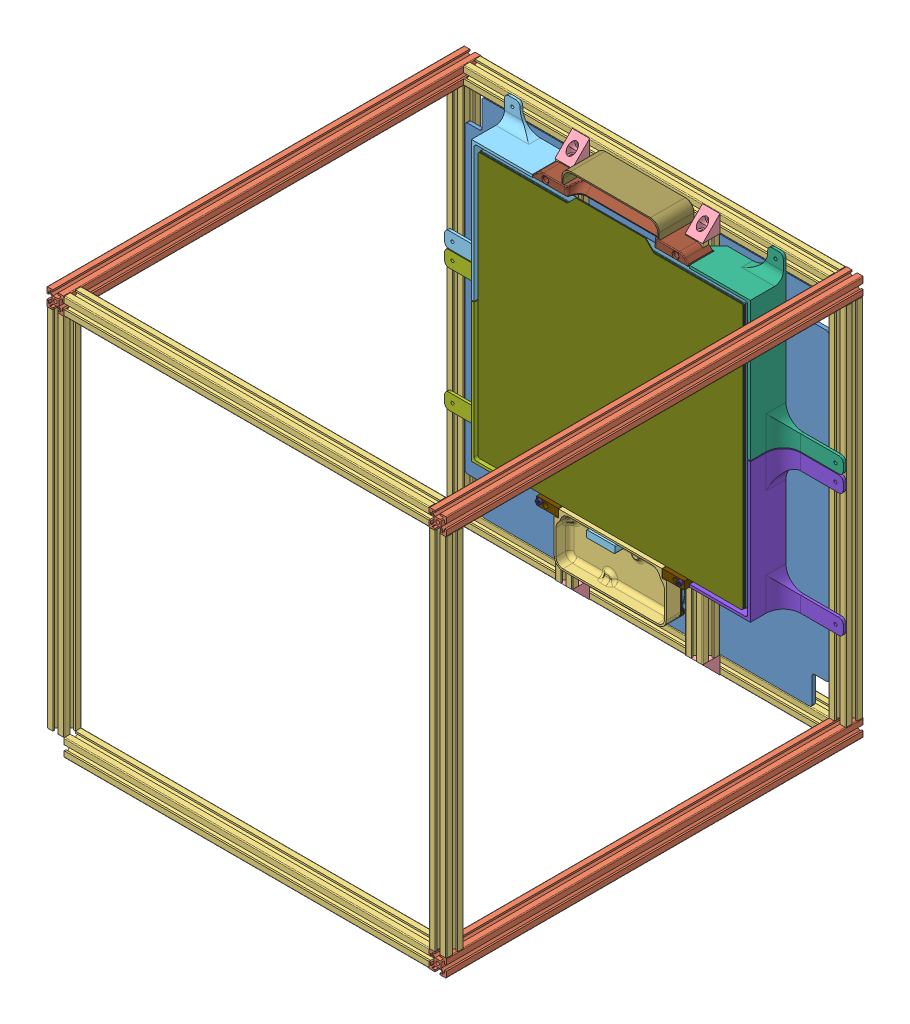
SolidWorks assembly Voron_full, configuration Default. Lengths in mm.
Overall size (460 460 480).
60 component instances, 23 part files, 98 mates.
Components (placement in the parent):
- bottom panel-1: bottom panel [Default] at (79.6442 547.5398 47.79) size (419 419 4)
- Misumi HFSB5-2020-480-1: Misumi HFSB5-2020-480 [Default] at (298.6442 327.5398 271.79) x (1 0 0) z (0 -1 0) size (20 480 20)
- Misumi HFSB5-2020-480-2: Misumi HFSB5-2020-480 [Default] at (-141.3558 327.5398 271.79) x (1 0 0) z (0 -1 0) size (20 480 20) (hidden)
- Misumi HFSB5-2020-480-3: Misumi HFSB5-2020-480 [Default] at (298.6442 767.5398 271.79) x (1 0 0) z (0 -1 0) size (20 480 20)
- Misumi HFSB5-2020-480-4: Misumi HFSB5-2020-480 [Default] at (-141.3558 767.5398 271.79) x (1 0 0) z (0 -1 0) size (20 480 20)
- Misumi HFSB5-2020-420-6: Misumi HFSB5-2020-420 [Default] at (-141.3558 547.5398 41.79) size (20 420 20)
- Misumi HFSB5-2020-420-8: Misumi HFSB5-2020-420 [Default] at (298.6442 547.5398 41.79) size (20 420 20)
- Misumi HFSB5-2020-420-10: Misumi HFSB5-2020-420 [Default] at (78.6442 327.5398 41.79) x (0 1 0) z (0 0 1) size (20 420 20)
- Misumi HFSB5-2020-420-12: Misumi HFSB5-2020-420 [Default] at (78.6442 767.5398 41.79) x (0 1 0) z (0 0 1) size (20 420 20)
- Misumi HFSB5-2020-420-7: Misumi HFSB5-2020-420 [Default] at (-141.3558 547.5398 501.79) size (20 420 20)
- Misumi HFSB5-2020-420-9: Misumi HFSB5-2020-420 [Default] at (298.6442 547.5398 501.79) size (20 420 20)
- Misumi HFSB5-2020-420-11: Misumi HFSB5-2020-420 [Default] at (78.6442 327.5398 501.79) x (0 1 0) z (0 0 1) size (20 420 20)
- Misumi HFSB5-2020-420-13: Misumi HFSB5-2020-420 [Default] at (78.6442 767.5398 501.79) x (0 1 0) z (0 0 1) size (20 420 20)
- Misumi HFSB5-2020-420-14: Misumi HFSB5-2020-420 [Default] at (153.6442 547.5398 61.79) size (20 420 20)
- Misumi HFSB5-2020-420-15: Misumi HFSB5-2020-420 [Default] at (3.6442 547.5398 61.79) size (20 420 20)
- OpenBuilds Billet Angle Corner Connector (2020)-1: OpenBuilds Billet Angle Corner Connector (2020) [Default] at (3.6442 757.5398 51.79) size (20 20 20)
- OpenBuilds Billet Angle Corner Connector (2020)-2: OpenBuilds Billet Angle Corner Connector (2020) [Default] at (153.6442 757.5398 51.79) size (20 20 20)
- OpenBuilds Billet Angle Corner Connector (2020)-3: OpenBuilds Billet Angle Corner Connector (2020) [Default] at (3.6442 337.5398 51.79) x (-1 0 0) z (0 0 1) size (20 20 20)
- OpenBuilds Billet Angle Corner Connector (2020)-4: OpenBuilds Billet Angle Corner Connector (2020) [Default] at (153.6442 337.5398 51.79) x (-1 0 0) z (0 0 1) size (20 20 20)
- Draft nozzle front side 1-3: Draft nozzle front side 1 [Default] at (-43.8558 669.5398 51.79) x (0 -1 0) z (0 0 1) size (187 149.5 41)
- Draft nozzle front side 2-2: Draft nozzle front side 2 [Default] at (277.1442 669.5398 51.79) x (0 -1 0) z (0 0 1) size (187 149.5 41)
- Draft nozzle back side 1-1: Draft nozzle back side 1 [Default] at (-43.8558 668.5398 51.79) x (0 -1 0) z (0 0 1) size (160 149.5 41)
- Draft nozzle back side 2-1: Draft nozzle back side 2 [Default] at (277.1442 668.5398 51.79) x (0 -1 0) z (0 0 1) size (160 149.5 41)
- Z-Stop LDO Mirrored-1: Z-Stop LDO Mirrored [Default] at (-16.3558 430.0398 68.79) x (0 1 0) z (0 0 -1) size (35 20.8 15.3)
- inner draft shield-1: inner draft shield [Default] at (78.6442 661.5398 51.79) x (-1 0 0) z (0 0 1) size (129 20 22)
- Draft nozzle front-3: Draft nozzle front [Default] at (78.6442 746.5398 72.04) x (-1 0 0) z (0 1 0) size (179 41.54 13.26)
- front_bucket-1: front_bucket [Default] at (78.6442 764.0398 51.79) x (-1 0 0) z (0 0 1) size (112 21 41)
- knurled nut-1: knurled nut [Default] at (154.1442 443.5398 73.7694) size (16 16 9.5)
- knurled nut-2: knurled nut [Default] at (154.1442 734.5398 73.7694) size (16 16 9.5)
- knurled nut-3: knurled nut [Default] at (4.1442 734.5398 73.7694) size (16 16 9.5)
- knurled nut-4: knurled nut [Default] at (4.1442 443.5398 73.7694) size (16 16 9.5)
- buildplate aluminium-1: buildplate aluminium [Default] at (79.1442 589.0398 81.29) size (305 305 10)
- Magnet sheet-1: Magnet sheet [Default] at (79.1442 589.0398 91.29) size (305 305 1.25)
- PEI sheet-1: PEI sheet [Default] at (79.1442 589.0398 92.54) x (-1 0 0) z (0 0 1) size (305 315 0.75)
- Blower_assembly-1: Blower_assembly [Default] at (-3.6341 431.5398 51.79) x (-1 0 0) z (0 0 1) size (170 62.88 44)
  - socket head cap screw_iso-1: socket head cap screw_iso [ISO 4762 M3 x 20 - 20N] at (-23.2783 15.4 23.5) x (0 0 -1) z (0.923728 0.383049 0) size (23 5.5 5.5)
  - socket head cap screw_iso-2: socket head cap screw_iso [ISO 4762 M3 x 20 - 20N] at (-98.2783 15.4 23.5) x (0 0 -1) z (0.923728 0.383049 0) size (23 5.5 5.5)
  - socket head cap screw_iso-3: socket head cap screw_iso [ISO 4762 M3 x 20 - 20N] at (-66.2783 53.4 23.5) x (0 0 -1) z (0.923728 0.383049 0) size (23 5.5 5.5)
  - socket head cap screw_iso-4: socket head cap screw_iso [ISO 4762 M3 x 20 - 20N] at (-141.2783 53.4 23.5) x (0 0 -1) z (0.923728 0.383049 0) size (23 5.5 5.5)
  - socket head cap screw_iso-5: socket head cap screw_iso [ISO 4762 M3 x 8 - 8N] at (-163.2783 2.75 44) x (0 0 -1) z (1 0 0) size (11 5.5 5.5)
  - socket head cap screw_iso-6: socket head cap screw_iso [ISO 4762 M3 x 8 - 8N] at (-1.2783 2.75 44) x (0 0 -1) z (1 0 0) size (11 5.5 5.5)
  - oven_back cover-1: oven_back cover [Default] at (-82.2783 0 22.7085) x (-1 0 0) z (0 1 0) size (170 41 59.3)
  - LDO Nevermore fan-1: LDO Nevermore fan [Default] at (-43.2783 33.4 3) x (0 1 0) z (0 0 1) size (52.88 55.98 18.27)
  - LDO Nevermore fan-2: LDO Nevermore fan [Default] at (-118.2783 33.4 3) x (0 1 0) z (0 0 1) size (52.88 55.98 18.27)
  - M3 heatset insert 3mm-1: M3 heatset insert 3mm [Default] at (-141.2783 53.4 0) size (4.55 4.55 3)
  - M3 heatset insert 3mm-2: M3 heatset insert 3mm [Default] at (-98.2783 15.4 0) size (4.55 4.55 3)
  - M3 heatset insert 3mm-3: M3 heatset insert 3mm [Default] at (-66.2783 53.4 0) size (4.55 4.55 3)
  - M3 heatset insert 3mm-4: M3 heatset insert 3mm [Default] at (-23.2783 15.4 0) size (4.55 4.55 3)
  - M3 heatset insert 3mm-5: M3 heatset insert 3mm [Default] at (-1.2783 2.75 38) size (4.55 4.55 3)
  - M3 heatset insert 3mm-6: M3 heatset insert 3mm [Default] at (-163.2783 2.75 38) size (4.55 4.55 3)
  - M3 heatset insert 3mm-7: M3 heatset insert 3mm [Default] at (-59.7783 3 33.5151) x (1 0 0) z (0 -1 0) size (4.55 4.55 3)
  - M3 heatset insert 3mm-8: M3 heatset insert 3mm [Default] at (-85.7783 3 33.5151) x (1 0 0) z (0 -1 0) size (4.55 4.55 3)
  - purge bucket-1: purge bucket [Default] at (-82.2783 15 24.2651) x (-1 0 0) z (0 0 1) size (129 59.3 17)
  - neodymium magnet 6x3mm-1: neodymium magnet 6x3mm [Default] at (-141.2783 53.4 24.2651) size (6 6 3)
  - neodymium magnet 6x3mm-2: neodymium magnet 6x3mm [Default] at (-98.2783 15.4 24.2651) size (6 6 3)
  - neodymium magnet 6x3mm-3: neodymium magnet 6x3mm [Default] at (-66.2783 53.4 24.2651) size (6 6 3)
  - neodymium magnet 6x3mm-4: neodymium magnet 6x3mm [Default] at (-23.2783 15.4 24.2651) size (6 6 3)
  - socket head cap screw_iso-7: socket head cap screw_iso [ISO 4762 M3 x 5 - 5N] at (-85.7783 6 33.5151) x (0 -1 0) z (-0.546944 0 0.837169) size (8 5.5 5.5)
  - socket head cap screw_iso-8: socket head cap screw_iso [ISO 4762 M3 x 5 - 5N] at (-59.7783 6 33.5151) x (0 -1 0) z (-0.546944 0 0.837169) size (8 5.5 5.5)
  - brush-1: brush [Default] at (-72.2783 7.5 25.2651) size (35 10 17)
Mates (geometry in assembly coordinates):
- Coincident1: coincident aligned: plane of Misumi HFSB5-2020-480-3 through (288.6442 777.5398 31.79) normal (0 1 0); plane of Misumi HFSB5-2020-480-4 through (-131.3558 777.5398 31.79) normal (0 1 0)
- Coincident2: coincident aligned: plane of Misumi HFSB5-2020-480-1 through (288.6442 337.5398 31.79) normal (0 1 0); plane of Misumi HFSB5-2020-480-2 through (-131.3558 337.5398 31.79) normal (0 1 0)
- Coincident3: coincident aligned: plane of Misumi HFSB5-2020-480-1 through (308.6442 317.5398 31.79) normal (1 0 0); plane of Misumi HFSB5-2020-480-3 through (308.6442 757.5398 31.79) normal (1 0 0)
- Coincident4: coincident aligned: plane of Misumi HFSB5-2020-480-1 through (298.6442 327.5398 511.79) normal (0 0 1); plane of Misumi HFSB5-2020-480-2 through (-141.3558 327.5398 511.79) normal (0 0 1)
- Coincident5: coincident aligned: plane of Misumi HFSB5-2020-480-1 through (298.6442 327.5398 511.79) normal (0 0 1); plane of Misumi HFSB5-2020-480-3 through (298.6442 767.5398 511.79) normal (0 0 1)
- Coincident6: coincident aligned: plane of Misumi HFSB5-2020-480-3 through (298.6442 767.5398 511.79) normal (0 0 1); plane of Misumi HFSB5-2020-480-4 through (-141.3558 767.5398 511.79) normal (0 0 1)
- Coincident7: coincident aligned: plane of Misumi HFSB5-2020-480-2 through (-131.3558 337.5398 31.79) normal (1 0 0); plane of Misumi HFSB5-2020-480-4 through (-131.3558 777.5398 31.79) normal (1 0 0)
- Coincident8: coincident aligned: plane of Misumi HFSB5-2020-420-7 through (-151.3558 337.5398 511.79) normal (0 0 1); plane of Misumi HFSB5-2020-420-9 through (288.6442 337.5398 511.79) normal (0 0 1)
- Coincident9: coincident aligned: plane of Misumi HFSB5-2020-420-7 through (-141.3558 757.5398 501.79) normal (0 1 0); plane of Misumi HFSB5-2020-420-9 through (298.6442 757.5398 501.79) normal (0 1 0)
- Coincident11: coincident aligned: plane of Misumi HFSB5-2020-420-7 through (-151.3558 337.5398 511.79) normal (0 0 1); plane of Misumi HFSB5-2020-420-11 through (288.6442 337.5398 511.79) normal (0 0 1)
- Coincident12: coincident anti-aligned: plane of Misumi HFSB5-2020-420-9 through (298.6442 337.5398 501.79) normal (0 -1 0); plane of Misumi HFSB5-2020-420-11 through (288.6442 337.5398 511.79) normal (0 1 0)
- Coincident13: coincident anti-aligned: plane of Misumi HFSB5-2020-420-7 through (-131.3558 337.5398 511.79) normal (1 0 0); plane of Misumi HFSB5-2020-420-11 through (-131.3558 327.5398 501.79) normal (-1 0 0)
- Coincident14: coincident anti-aligned: plane of Misumi HFSB5-2020-420-9 through (288.6442 337.5398 511.79) normal (-1 0 0); plane of Misumi HFSB5-2020-420-11 through (288.6442 327.5398 501.79) normal (1 0 0)
- Coincident15: coincident aligned: plane of Misumi HFSB5-2020-420-11 through (288.6442 327.5398 501.79) normal (1 0 0); plane of Misumi HFSB5-2020-420-13 through (288.6442 767.5398 501.79) normal (1 0 0)
- Coincident16: coincident aligned: plane of Misumi HFSB5-2020-420-9 through (288.6442 337.5398 511.79) normal (0 0 1); plane of Misumi HFSB5-2020-420-13 through (288.6442 777.5398 511.79) normal (0 0 1)
- Coincident17: coincident anti-aligned: plane of Misumi HFSB5-2020-420-9 through (298.6442 757.5398 501.79) normal (0 1 0); plane of Misumi HFSB5-2020-420-13 through (288.6442 757.5398 511.79) normal (0 -1 0)
- Coincident18: coincident aligned: plane of Misumi HFSB5-2020-480-1 through (298.6442 327.5398 511.79) normal (0 0 1); plane of Misumi HFSB5-2020-420-9 through (288.6442 337.5398 511.79) normal (0 0 1)
- Coincident19: coincident anti-aligned: plane of Misumi HFSB5-2020-480-1 through (288.6442 337.5398 31.79) normal (0 1 0); plane of Misumi HFSB5-2020-420-9 through (298.6442 337.5398 501.79) normal (0 -1 0)
- Coincident20: coincident anti-aligned: plane of Misumi HFSB5-2020-480-1 through (288.6442 317.5398 31.79) normal (-1 0 0); plane of Misumi HFSB5-2020-420-11 through (288.6442 327.5398 501.79) normal (1 0 0)
- Coincident21: coincident anti-aligned: plane of Misumi HFSB5-2020-480-2 through (-131.3558 317.5398 31.79) normal (1 0 0); plane of Misumi HFSB5-2020-420-11 through (-131.3558 327.5398 501.79) normal (-1 0 0)
- Coincident22: coincident anti-aligned: plane of Misumi HFSB5-2020-480-4 through (-151.3558 757.5398 31.79) normal (0 -1 0); plane of Misumi HFSB5-2020-420-7 through (-141.3558 757.5398 501.79) normal (0 1 0)
- Coincident23: coincident aligned: plane of Misumi HFSB5-2020-420-6 through (-151.3558 337.5398 51.79) normal (0 0 1); plane of Misumi HFSB5-2020-420-10 through (288.6442 337.5398 51.79) normal (0 0 1)
- Coincident24: coincident aligned: plane of Misumi HFSB5-2020-420-8 through (308.6442 337.5398 51.79) normal (0 0 1); plane of Misumi HFSB5-2020-420-10 through (288.6442 337.5398 51.79) normal (0 0 1)
- Coincident25: coincident aligned: plane of Misumi HFSB5-2020-420-6 through (-141.3558 337.5398 41.79) normal (0 -1 0); plane of Misumi HFSB5-2020-420-8 through (298.6442 337.5398 41.79) normal (0 -1 0)
- Coincident26: coincident anti-aligned: plane of Misumi HFSB5-2020-420-6 through (-141.3558 337.5398 41.79) normal (0 -1 0); plane of Misumi HFSB5-2020-420-10 through (288.6442 337.5398 51.79) normal (0 1 0)
- Coincident27: coincident aligned: plane of Misumi HFSB5-2020-420-6 through (-151.3558 337.5398 51.79) normal (0 0 1); plane of Misumi HFSB5-2020-420-12 through (288.6442 757.5398 51.79) normal (0 0 1)
- Coincident28: coincident aligned: plane of Misumi HFSB5-2020-420-10 through (-131.3558 327.5398 41.79) normal (-1 0 0); plane of Misumi HFSB5-2020-420-12 through (-131.3558 767.5398 41.79) normal (-1 0 0)
- Coincident29: coincident anti-aligned: plane of Misumi HFSB5-2020-420-6 through (-131.3558 337.5398 51.79) normal (1 0 0); plane of Misumi HFSB5-2020-420-10 through (-131.3558 327.5398 41.79) normal (-1 0 0)
- Coincident30: coincident anti-aligned: plane of Misumi HFSB5-2020-420-6 through (-141.3558 757.5398 41.79) normal (0 1 0); plane of Misumi HFSB5-2020-420-12 through (288.6442 757.5398 51.79) normal (0 -1 0)
- Coincident31: coincident anti-aligned: plane of Misumi HFSB5-2020-420-8 through (288.6442 337.5398 51.79) normal (-1 0 0); plane of Misumi HFSB5-2020-420-10 through (288.6442 327.5398 41.79) normal (1 0 0)
- Coincident32: coincident aligned: plane of Misumi HFSB5-2020-480-2 through (-141.3558 327.5398 31.79) normal (0 0 -1); plane of Misumi HFSB5-2020-420-6 through (-151.3558 337.5398 31.79) normal (0 0 -1)
- Coincident33: coincident anti-aligned: plane of Misumi HFSB5-2020-480-2 through (-151.3558 337.5398 31.79) normal (0 1 0); plane of Misumi HFSB5-2020-420-6 through (-141.3558 337.5398 41.79) normal (0 -1 0)
- Coincident34: coincident anti-aligned: plane of Misumi HFSB5-2020-480-2 through (-131.3558 317.5398 31.79) normal (1 0 0); plane of Misumi HFSB5-2020-420-10 through (-131.3558 327.5398 41.79) normal (-1 0 0)
- Coincident35: coincident aligned: plane of Misumi HFSB5-2020-420-14 through (143.6442 337.5398 71.79) normal (0 0 1); plane of Misumi HFSB5-2020-420-15 through (13.6442 337.5398 71.79) normal (0 0 1)
- Coincident36: coincident aligned: plane of Misumi HFSB5-2020-420-14 through (153.6442 757.5398 61.79) normal (0 1 0); plane of Misumi HFSB5-2020-420-15 through (3.6442 757.5398 61.79) normal (0 1 0)
- Coincident37: coincident anti-aligned: plane of Misumi HFSB5-2020-420-12 through (288.6442 757.5398 51.79) normal (0 -1 0); plane of Misumi HFSB5-2020-420-14 through (153.6442 757.5398 61.79) normal (0 1 0)
- Coincident38: coincident anti-aligned: plane of Misumi HFSB5-2020-420-12 through (288.6442 757.5398 51.79) normal (0 0 1); plane of Misumi HFSB5-2020-420-14 through (143.6442 337.5398 51.79) normal (0 0 -1)
- Distance1: distance = 130 mm anti-aligned: plane of Misumi HFSB5-2020-420-15 through (13.6442 337.5398 71.79) normal (1 0 0); plane of Misumi HFSB5-2020-420-14 through (143.6442 337.5398 71.79) normal (-1 0 0)
- Distance2: distance = 125 mm anti-aligned: plane of Misumi HFSB5-2020-420-14 through (163.6442 337.5398 51.79) normal (1 0 0); plane of Misumi HFSB5-2020-420-8 through (288.6442 337.5398 51.79) normal (-1 0 0)
- Coincident42: coincident aligned: plane of OpenBuilds Billet Angle Corner Connector (2020)-3 through (13.6442 337.5398 51.79) normal (0 1 0); plane of OpenBuilds Billet Angle Corner Connector (2020)-4 through (163.6442 337.5398 51.79) normal (0 1 0)
- Coincident43: coincident aligned: plane of OpenBuilds Billet Angle Corner Connector (2020)-3 through (13.6442 337.5398 51.79) normal (0 0 -1); plane of OpenBuilds Billet Angle Corner Connector (2020)-4 through (163.6442 337.5398 51.79) normal (0 0 -1)
- Coincident44: coincident aligned: plane of OpenBuilds Billet Angle Corner Connector (2020)-1 through (-6.3558 757.5398 51.79) normal (0 0 -1); plane of OpenBuilds Billet Angle Corner Connector (2020)-2 through (143.6442 757.5398 51.79) normal (0 0 -1)
- Coincident45: coincident aligned: plane of OpenBuilds Billet Angle Corner Connector (2020)-1 through (-6.3558 757.5398 51.79) normal (0 -1 0); plane of OpenBuilds Billet Angle Corner Connector (2020)-2 through (143.6442 757.5398 51.79) normal (0 -1 0)
- Coincident46: coincident aligned: plane of OpenBuilds Billet Angle Corner Connector (2020)-2 through (143.6442 757.5398 51.79) normal (0 0 -1); plane of OpenBuilds Billet Angle Corner Connector (2020)-4 through (163.6442 337.5398 51.79) normal (0 0 -1)
- Coincident47: coincident aligned: plane of Misumi HFSB5-2020-420-14 through (143.6442 337.5398 51.79) normal (0 0 -1); plane of OpenBuilds Billet Angle Corner Connector (2020)-4 through (163.6442 337.5398 51.79) normal (0 0 -1)
- Coincident48: coincident anti-aligned: plane of Misumi HFSB5-2020-420-14 through (153.6442 757.5398 61.79) normal (0 1 0); plane of OpenBuilds Billet Angle Corner Connector (2020)-2 through (143.6442 757.5398 51.79) normal (0 -1 0)
- Coincident49: coincident anti-aligned: plane of Misumi HFSB5-2020-420-14 through (153.6442 337.5398 61.79) normal (0 -1 0); plane of OpenBuilds Billet Angle Corner Connector (2020)-4 through (163.6442 337.5398 51.79) normal (0 1 0)
- Coincident50: coincident aligned: plane of OpenBuilds Billet Angle Corner Connector (2020)-2 through (163.6442 757.5398 51.79) normal (1 0 0); plane of OpenBuilds Billet Angle Corner Connector (2020)-4 through (163.6442 337.5398 51.79) normal (1 0 0)
- Coincident51: coincident aligned: plane of Misumi HFSB5-2020-420-14 through (163.6442 337.5398 71.79) normal (1 0 0); plane of OpenBuilds Billet Angle Corner Connector (2020)-2 through (163.6442 757.5398 51.79) normal (1 0 0)
- Coincident52: coincident aligned: plane of Misumi HFSB5-2020-420-15 through (13.6442 337.5398 51.79) normal (1 0 0); plane of OpenBuilds Billet Angle Corner Connector (2020)-1 through (13.6442 757.5398 51.79) normal (1 0 0)
- Coincident53: coincident aligned: plane of OpenBuilds Billet Angle Corner Connector (2020)-1 through (13.6442 757.5398 51.79) normal (1 0 0); plane of OpenBuilds Billet Angle Corner Connector (2020)-3 through (13.6442 337.5398 51.79) normal (1 0 0)
- Coincident54: coincident aligned: plane of knurled nut-1 through (154.1442 447.5398 76.29) normal (0 0 1); plane of knurled nut-2 through (154.1442 738.5398 76.29) normal (0 0 1)
- Coincident55: coincident aligned: plane of knurled nut-2 through (154.1442 738.5398 76.29) normal (0 0 1); plane of knurled nut-3 through (4.1442 738.5398 76.29) normal (0 0 1)
- Coincident56: coincident anti-aligned: circle of knurled nut-3; plane of knurled nut-4 through (4.1442 447.5398 76.29) normal (0 0 1)
- Coincident57: coincident anti-aligned: plane of Misumi HFSB5-2020-420-14 through (143.6442 337.5398 71.79) normal (0 0 1); plane of knurled nut-4 through (4.1442 451.5398 71.79) normal (0 0 -1)
- Coincident58: coincident anti-aligned: plane of knurled nut-3 through (4.1442 735.7898 81.29) normal (0 0 1); plane of buildplate aluminium-1 through (79.1442 589.0398 81.29) normal (0 0 -1)
- Distance3: distance = 58 mm anti-aligned: plane of buildplate aluminium-1 through (-73.3558 436.5398 91.29) normal (-1 0 0); plane of Misumi HFSB5-2020-480-4 through (-131.3558 757.5398 31.79) normal (1 0 0)
- Concentric1: concentric anti-aligned: cylinder of knurled nut-2 through (154.1442 734.5398 73.7694) axis (0 0 -1) radius 1.25; cylinder of buildplate aluminium-1 through (154.1442 734.5398 81.29) axis (0 0 1) radius 1.7
- Concentric2: concentric anti-aligned: cylinder of knurled nut-3 through (4.1442 734.5398 73.7694) axis (0 0 -1) radius 1.25; cylinder of buildplate aluminium-1 through (4.1442 734.5398 81.29) axis (0 0 1) radius 1.7
- Concentric3: concentric anti-aligned: cylinder of knurled nut-4 through (4.1442 443.5398 73.7694) axis (0 0 -1) radius 1.25; circle of buildplate aluminium-1
- Concentric4: concentric anti-aligned: cylinder of knurled nut-1 through (154.1442 443.5398 73.7694) axis (0 0 -1) radius 1.25; cylinder of buildplate aluminium-1 through (154.1442 443.5398 81.29) axis (0 0 1) radius 1.7
- Coincident60: coincident anti-aligned: plane of buildplate aluminium-1 through (79.1442 589.0398 91.29) normal (0 0 1); plane of Magnet sheet-1 through (79.1442 589.0398 91.29) normal (0 0 -1)
- Coincident61: coincident aligned: plane of buildplate aluminium-1 through (-73.3558 741.5398 91.29) normal (0 1 0); plane of Magnet sheet-1 through (-73.3558 741.5398 92.54) normal (0 1 0)
- Coincident62: coincident aligned: plane of buildplate aluminium-1 through (231.6442 436.5398 91.29) normal (1 0 0); plane of Magnet sheet-1 through (231.6442 741.5398 92.54) normal (1 0 0)
- Coincident63: coincident anti-aligned: plane of Magnet sheet-1 through (79.1442 589.0398 92.54) normal (0 0 1); plane of PEI sheet-1 through (79.1442 589.0398 92.54) normal (0 0 -1)
- Coincident64: coincident aligned: plane of buildplate aluminium-1 through (-73.3558 741.5398 91.29) normal (0 1 0); plane of PEI sheet-1 through (231.6442 741.5398 93.29) normal (0 1 0)
- Coincident65: coincident aligned: plane of buildplate aluminium-1 through (231.6442 436.5398 91.29) normal (1 0 0); plane of PEI sheet-1 through (231.6442 741.5398 93.29) normal (1 0 0)
- Distance4: distance = 16 mm aligned: plane of buildplate aluminium-1 through (-73.3558 741.5398 91.29) normal (0 1 0); plane of Misumi HFSB5-2020-420-15 through (3.6442 757.5398 61.79) normal (0 1 0)
- Coincident67: coincident anti-aligned: plane of Misumi HFSB5-2020-420-14 through (163.6442 337.5398 51.79) normal (0 0 -1); plane of bottom panel-1 through (79.6442 547.5398 51.79) normal (0 0 1)
- Distance5: distance = 0.5 mm anti-aligned: plane of bottom panel-1 through (289.1442 338.0398 51.79) normal (1 0 0); plane of Misumi HFSB5-2020-420-8 through (288.6442 337.5398 31.79) normal (-1 0 0)
- Distance6: distance = 0.5 mm anti-aligned: plane of bottom panel-1 through (-129.8558 338.0398 51.79) normal (0 -1 0); plane of Misumi HFSB5-2020-420-10 through (288.6442 337.5398 51.79) normal (0 1 0)
- Coincident72: coincident anti-aligned: plane of bottom panel-1 through (79.6442 547.5398 51.79) normal (0 0 1); plane of Draft nozzle front side 1-3 through (-43.8558 669.5398 51.79) normal (0 0 -1)
- Distance7: distance = 5 mm anti-aligned: plane of Draft nozzle front side 1-3 through (-78.3558 589.5398 92.79) normal (1 0 0); plane of buildplate aluminium-1 through (-73.3558 436.5398 91.29) normal (-1 0 0)
- Distance8: distance = 5 mm anti-aligned: plane of Draft nozzle front side 1-3 through (-78.3558 746.5398 92.79) normal (0 -1 0); plane of buildplate aluminium-1 through (-73.3558 741.5398 91.29) normal (0 1 0)
- Coincident75: coincident anti-aligned: plane of bottom panel-1 through (79.6442 547.5398 51.79) normal (0 0 1); plane of Draft nozzle front side 2-2 through (202.1442 669.5398 51.79) normal (0 0 -1)
- Distance9: distance = 5 mm anti-aligned: plane of Draft nozzle front side 2-2 through (236.6442 589.5398 92.79) normal (-1 0 0); plane of buildplate aluminium-1 through (231.6442 436.5398 91.29) normal (1 0 0)
- Coincident77: coincident aligned: plane of Draft nozzle front side 1-3 through (-81.3558 749.5398 54.79) normal (0 1 0); plane of Draft nozzle front side 2-2 through (239.6442 749.5398 54.79) normal (0 1 0)
- Coincident79: coincident aligned: plane of Draft nozzle front side 1-3 through (-81.3558 749.5398 54.79) normal (-1 0 0); plane of Draft nozzle back side 1-1 through (-81.3558 428.5398 54.79) normal (-1 0 0)
- Coincident80: coincident anti-aligned: plane of bottom panel-1 through (79.6442 547.5398 51.79) normal (0 0 1); plane of Draft nozzle back side 1-1 through (-43.8558 508.5398 51.79) normal (0 0 -1)
- Distance12: distance = 5 mm anti-aligned: plane of Draft nozzle back side 1-1 through (-78.3558 431.5398 92.79) normal (0 1 0); plane of buildplate aluminium-1 through (-73.3558 436.5398 91.29) normal (0 -1 0)
- Coincident82: coincident anti-aligned: plane of bottom panel-1 through (79.6442 547.5398 51.79) normal (0 0 1); plane of Draft nozzle back side 2-1 through (202.1442 508.5398 51.79) normal (0 0 -1)
- Coincident83: coincident aligned: plane of Draft nozzle front side 2-2 through (239.6442 749.5398 54.79) normal (1 0 0); plane of Draft nozzle back side 2-1 through (239.6442 428.5398 54.79) normal (1 0 0)
- Distance13: distance = 5 mm anti-aligned: plane of Draft nozzle back side 2-1 through (236.6442 431.5398 92.79) normal (0 1 0); plane of buildplate aluminium-1 through (-73.3558 436.5398 91.29) normal (0 -1 0)
- Coincident90: coincident anti-aligned: plane of Misumi HFSB5-2020-420-15 through (-6.3558 337.5398 71.79) normal (-1 0 0); plane of Z-Stop LDO Mirrored-1 through (-6.3558 412.5398 53.49) normal (1 0 0)
- Distance15: distance = 3 mm aligned: plane of Z-Stop LDO Mirrored-1 through (-16.3558 430.0398 68.79) normal (0 0 1); plane of Misumi HFSB5-2020-420-15 through (-6.3558 337.5398 71.79) normal (0 0 1)
- Distance16: distance = 0.5 mm anti-aligned: plane of Z-Stop LDO Mirrored-1 through (-26.3558 447.5398 53.49) normal (0 1 0); plane of Draft nozzle back side 1-1 through (-43.8558 448.0398 51.79) normal (0 -1 0)
- Parallel1: parallel anti-aligned: plane of Misumi HFSB5-2020-420-14 through (143.6442 337.5398 71.79) normal (0 0 1); plane of Blower_assembly-1/oven_back cover-1 through (163.6442 422.5398 72.29) normal (0 0 -1)
- Distance17: distance = 0.5 mm anti-aligned: plane of Blower_assembly-1/oven_back cover-1 through (143.1442 422.5398 51.79) normal (1 0 0); plane of Misumi HFSB5-2020-420-14 through (143.6442 337.5398 71.79) normal (-1 0 0)
- Coincident93: coincident anti-aligned: plane of bottom panel-1 through (79.6442 547.5398 51.79) normal (0 0 1); plane of Blower_assembly-1/oven_back cover-1 through (14.1442 422.5398 51.79) normal (0 0 -1)
- Coincident94: coincident aligned: plane of Draft nozzle back side 2-1 through (236.6442 431.5398 92.79) normal (0 1 0); plane of Blower_assembly-1/oven_back cover-1 through (78.6442 431.5398 74.4985) normal (0 1 0)
- Coincident95: coincident anti-aligned: plane of bottom panel-1 through (79.6442 547.5398 51.79) normal (0 0 1); plane of inner draft shield-1 through (78.6442 661.5398 51.79) normal (0 0 -1)
- Distance18: distance = 0.5 mm anti-aligned: plane of inner draft shield-1 through (14.1442 651.5398 73.79) normal (-1 0 0); plane of Misumi HFSB5-2020-420-15 through (13.6442 337.5398 51.79) normal (1 0 0)
- Coincident99: coincident anti-aligned: plane of Misumi HFSB5-2020-420-14 through (163.6442 337.5398 71.79) normal (0 0 1); plane of Draft nozzle front-3 through (143.1442 756.5398 71.79) normal (0 0 -1)
- Coincident100: coincident aligned: plane of Draft nozzle front side 2-2 through (236.6442 746.5398 92.79) normal (0 -1 0); plane of Draft nozzle front-3 through (78.6442 746.5398 72.04) normal (0 -1 0)
- Distance20: distance = 0.5 mm anti-aligned: plane of Draft nozzle front-3 through (14.1442 756.5398 71.79) normal (-1 0 0); plane of Misumi HFSB5-2020-420-15 through (13.6442 337.5398 71.79) normal (1 0 0)
- Coincident102: coincident anti-aligned: plane of Draft nozzle front-3 through (78.6442 753.5398 72.04) normal (0 1 0); plane of front_bucket-1 through (134.6442 753.5398 92.79) normal (0 -1 0)
- Coincident103: coincident: line of Draft nozzle front-3 through (134.6442 756.5398 72.29) axis (0 0 -1); plane of front_bucket-1 through (134.6442 774.5398 92.79) normal (1 0 0)
- Coincident104: coincident aligned: plane of Draft nozzle front-3 through (128.6442 756.5398 92.79) normal (0 0 1); plane of front_bucket-1 through (78.6442 764.0398 92.79) normal (0 0 1)
